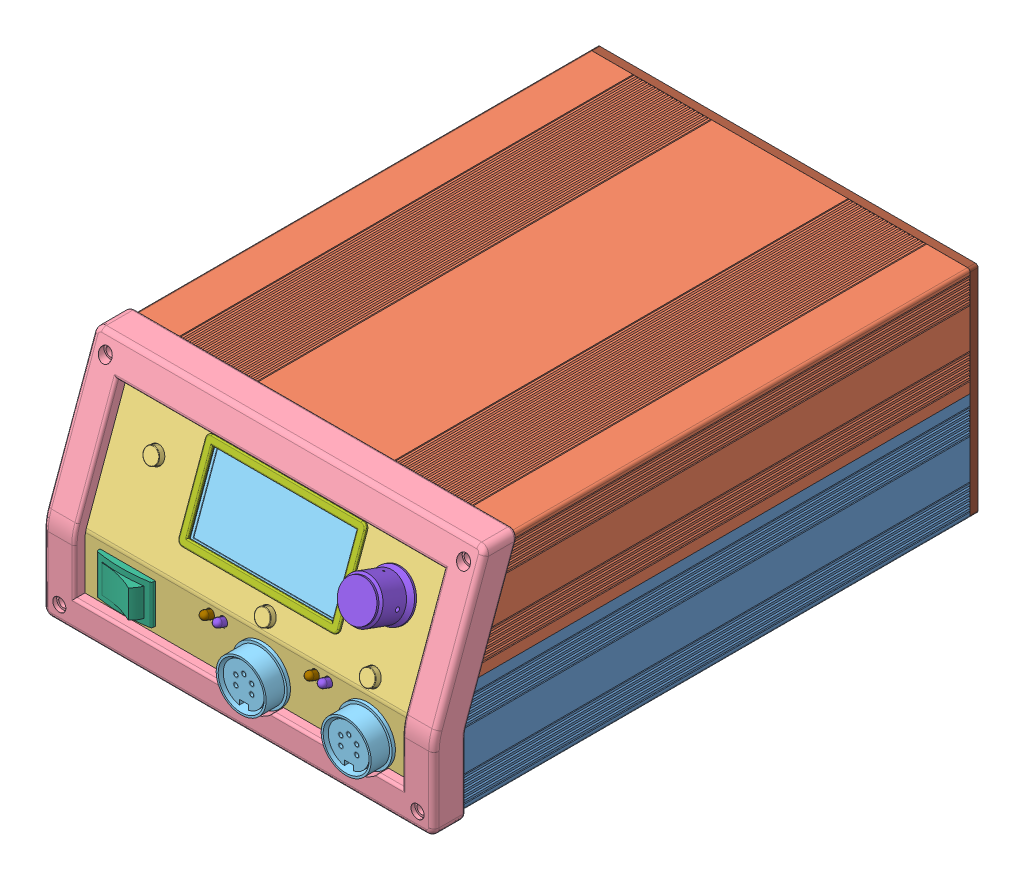
SolidWorks assembly Assembly, configuration Default. Lengths in mm. (continued)
Components (placement in the parent): (continued)
- SolderingStation-3: SolderingStation [Default] at (108 -45.1633 3.8854) x (-1 0 0) z (0 -0.34202 -0.939693) size (142.21 62 43.76) (continued)
  - SolderingStation.step-1: SolderingStation.step [Default] at origin size (142.21 62 43.76) (continued)
    - R10_ss.step-1: R10_ss.step [Default] at origin size (1.7 0.8 0.56)
      - User_Library-RES_1609-0603.step-1: User_Library-RES_1609-0603.step [Default] at (120.9541 53.774 0) x (1 0 0) z (0 -1 0) size (1.7 0.56 0.8)
    - R11_ss.step-1: R11_ss.step [Default] at origin size (0.8 1.7 0.56)
      - User_Library-RES_1609-0603.step-1: User_Library-RES_1609-0603.step [Default] at (79.298 51.2339 0) x (0 -1 0) z (-1 0 0) size (1.7 0.56 0.8)
    - R12_ss.step-1: R12_ss.step [Default] at origin size (0.8 1.7 0.56)
      - User_Library-RES_1609-0603.step-1: User_Library-RES_1609-0603.step [Default] at (118.7951 51.2339 0) x (0 -1 0) z (-1 0 0) size (1.7 0.56 0.8)
    - U3_ss.step-1: U3_ss.step [Default] at origin size (6.2 5 1.75)
      - User_Library-SOIC8_JEDEC_MS-012AA.step-1: User_Library-SOIC8_JEDEC_MS-012AA.step [Default] at (86.8348 63.0449 0) x (0 -1 0) z (-1 0 0) size (5 1.75 6.2)
    - C8_ss.step-1: C8_ss.step [Default] at origin size (1.6 0.8 0.3)
      - User_Library-0603_SMD_Capacitor.step-1: User_Library-0603_SMD_Capacitor.step [Default] at (89.7629 66.4487 0) x (1 0 0) z (0 -1 0) size (1.6 0.3 0.8)
    - C10_ss.step-1: C10_ss.step [Default] at origin size (1.6 0.8 0.3)
      - User_Library-0603_SMD_Capacitor.step-1: User_Library-0603_SMD_Capacitor.step [Default] at (85.2671 59.4891 0) x (1 0 0) z (0 -1 0) size (1.6 0.3 0.8)
    - D7_ss.step-1: D7_ss.step [Default] at origin size (2.5 3 1.1)
      - CircuitWorks-SOT-23.step-1: CircuitWorks-SOT-23.step [Default] at (79.4249 63.6799 0.5) x (0 -1 0) z (-1 0 0) size (3 1.1 2.5)
    - D3_ss.step-1: D3_ss.step [Default] at origin size (3 2.5 1.1)
      - CircuitWorks-SOT-23.step-1: CircuitWorks-SOT-23.step [Default] at (93.9031 63.8069 0.5) x (1 0 0) z (0 -1 0) size (3 1.1 2.5)
    - R13_ss.step-1: R13_ss.step [Default] at origin size (1.7 0.8 0.56)
      - User_Library-RES_1609-0603.step-1: User_Library-RES_1609-0603.step [Default] at (93.7759 66.474 0) x (-1 0 0) z (0 1 0) size (1.7 0.56 0.8)
    - R15_ss.step-1: R15_ss.step [Default] at origin size (0.8 1.7 0.56)
      - User_Library-RES_1609-0603.step-1: User_Library-RES_1609-0603.step [Default] at (96.57 65.7121 0) x (0 1 0) z (1 0 0) size (1.7 0.56 0.8)
    - R17_ss.step-1: R17_ss.step [Default] at origin size (0.8 1.7 0.56)
      - User_Library-RES_1609-0603.step-1: User_Library-RES_1609-0603.step [Default] at (96.57 62.7911 0) x (0 1 0) z (1 0 0) size (1.7 0.56 0.8)
    - R21_ss.step-1: R21_ss.step [Default] at origin size (0.8 1.7 0.56)
      - User_Library-RES_1609-0603.step-1: User_Library-RES_1609-0603.step [Default] at (91.1352 60.5051 0) x (0 1 0) z (1 0 0) size (1.7 0.56 0.8)
    - R22_ss.step-1: R22_ss.step [Default] at origin size (0.8 1.7 0.56)
      - User_Library-RES_1609-0603.step-1: User_Library-RES_1609-0603.step [Default] at (91.1352 63.0451 0) x (0 1 0) z (1 0 0) size (1.7 0.56 0.8)
    - R29_ss.step-1: R29_ss.step [Default] at origin size (1.7 0.8 0.56)
      - User_Library-RES_1609-0603.step-1: User_Library-RES_1609-0603.step [Default] at (79.8061 59.235 0) x (1 0 0) z (0 -1 0) size (1.7 0.56 0.8)
    - R31_ss.step-1: R31_ss.step [Default] at origin size (1.7 0.8 0.56)
      - User_Library-RES_1609-0603.step-1: User_Library-RES_1609-0603.step [Default] at (79.8061 60.632 0) x (1 0 0) z (0 -1 0) size (1.7 0.56 0.8)
    - R33_ss.step-1: R33_ss.step [Default] at origin size (0.8 1.7 0.56)
      - User_Library-RES_1609-0603.step-1: User_Library-RES_1609-0603.step [Default] at (82.0919 64.3151 0) x (0 1 0) z (1 0 0) size (1.7 0.56 0.8)
    - R35_ss.step-1: R35_ss.step [Default] at origin size (0.8 1.7 0.56)
      - User_Library-RES_1609-0603.step-1: User_Library-RES_1609-0603.step [Default] at (82.0919 61.7751 0) x (0 1 0) z (1 0 0) size (1.7 0.56 0.8)
    - R36_ss.step-1: R36_ss.step [Default] at origin size (0.8 1.7 0.56)
      - User_Library-RES_1609-0603.step-1: User_Library-RES_1609-0603.step [Default] at (121.97 61.7751 0) x (0 1 0) z (1 0 0) size (1.7 0.56 0.8)
    - R34_ss.step-1: R34_ss.step [Default] at origin size (0.8 1.7 0.56)
      - User_Library-RES_1609-0603.step-1: User_Library-RES_1609-0603.step [Default] at (121.97 64.3151 0) x (0 1 0) z (1 0 0) size (1.7 0.56 0.8)
    - R32_ss.step-1: R32_ss.step [Default] at origin size (1.7 0.8 0.56)
      - User_Library-RES_1609-0603.step-1: User_Library-RES_1609-0603.step [Default] at (119.8061 60.632 0) x (1 0 0) z (0 -1 0) size (1.7 0.56 0.8)
    - R30_ss.step-1: R30_ss.step [Default] at origin size (1.7 0.8 0.56)
      - User_Library-RES_1609-0603.step-1: User_Library-RES_1609-0603.step [Default] at (119.8061 59.235 0) x (1 0 0) z (0 -1 0) size (1.7 0.56 0.8)
    - R24_ss.step-1: R24_ss.step [Default] at origin size (0.8 1.7 0.56)
      - User_Library-RES_1609-0603.step-1: User_Library-RES_1609-0603.step [Default] at (131.0836 63.0451 0) x (0 1 0) z (1 0 0) size (1.7 0.56 0.8)
    - R23_ss.step-1: R23_ss.step [Default] at origin size (0.8 1.7 0.56)
      - User_Library-RES_1609-0603.step-1: User_Library-RES_1609-0603.step [Default] at (131.0885 60.5051 0) x (0 1 0) z (1 0 0) size (1.7 0.56 0.8)
    - R18_ss.step-1: R18_ss.step [Default] at origin size (0.8 1.7 0.56)
      - User_Library-RES_1609-0603.step-1: User_Library-RES_1609-0603.step [Default] at (136.5699 62.7911 0) x (0 1 0) z (1 0 0) size (1.7 0.56 0.8)
    - R16_ss.step-1: R16_ss.step [Default] at origin size (0.8 1.7 0.56)
      - User_Library-RES_1609-0603.step-1: User_Library-RES_1609-0603.step [Default] at (136.5699 65.7121 0) x (0 1 0) z (1 0 0) size (1.7 0.56 0.8)
    - R14_ss.step-1: R14_ss.step [Default] at origin size (1.7 0.8 0.56)
      - User_Library-RES_1609-0603.step-1: User_Library-RES_1609-0603.step [Default] at (133.7759 66.474 0) x (-1 0 0) z (0 1 0) size (1.7 0.56 0.8)
    - D4_ss.step-1: D4_ss.step [Default] at origin size (3 2.5 1.1)
      - CircuitWorks-SOT-23.step-1: CircuitWorks-SOT-23.step [Default] at (133.9031 63.8069 0.5) x (1 0 0) z (0 -1 0) size (3 1.1 2.5)
    - D8_ss.step-1: D8_ss.step [Default] at origin size (2.5 3 1.1)
      - CircuitWorks-SOT-23.step-1: CircuitWorks-SOT-23.step [Default] at (119.4299 63.6799 0.5) x (0 -1 0) z (-1 0 0) size (3 1.1 2.5)
    - C11_ss.step-1: C11_ss.step [Default] at origin size (1.6 0.8 0.3)
      - User_Library-0603_SMD_Capacitor.step-1: User_Library-0603_SMD_Capacitor.step [Default] at (125.2671 59.4891 0) x (1 0 0) z (0 -1 0) size (1.6 0.3 0.8)
    - C9_ss.step-1: C9_ss.step [Default] at origin size (1.6 0.8 0.3)
      - User_Library-0603_SMD_Capacitor.step-1: User_Library-0603_SMD_Capacitor.step [Default] at (129.6917 66.7027 0) x (1 0 0) z (0 -1 0) size (1.6 0.3 0.8)
    - U4_ss.step-1: U4_ss.step [Default] at origin size (6.2 5 1.75)
      - User_Library-SOIC8_JEDEC_MS-012AA.step-1: User_Library-SOIC8_JEDEC_MS-012AA.step [Default] at (126.8348 63.0449 0) x (0 -1 0) z (-1 0 0) size (5 1.75 6.2)
    - R44_ss.step-1: R44_ss.step [Default] at origin size (1.7 0.8 0.56)
      - User_Library-RES_1609-0603.step-1: User_Library-RES_1609-0603.step [Default] at (63.6769 67.1089 0) x (-1 0 0) z (0 1 0) size (1.7 0.56 0.8)
    - R46_ss.step-1: R46_ss.step [Default] at origin size (1.7 0.8 0.56)
      - User_Library-RES_1609-0603.step-1: User_Library-RES_1609-0603.step [Default] at (60.2481 67.109 0) x (1 0 0) z (0 -1 0) size (1.7 0.56 0.8)
    - FB1_ss.step-1: FB1_ss.step [Default] at origin size (1.25 2 0.85)
      - FB-0805.step-1: FB-0805.step [Default] at (55.5489 42.9791 0) x (0 1 0) z (0 0 1) size (2 1.25 0.85)
        - User_Library-FB_2012-1_Pad001.step-1: User_Library-FB_2012-1_Pad001.step [Default] at (0 0 0.03) size (1.94 1.19 0.79)
        - User_Library-FB_2012-1_Cut.step-1: User_Library-FB_2012-1_Cut.step [Default] at origin size (2 1.25 0.85)
    - FB2_ss.step-1: FB2_ss.step [Default] at origin size (1.25 2 0.85)
      - FB-0805.step-1: FB-0805.step [Default] at (95.6809 42.9791 0) x (0 1 0) z (0 0 1) size (2 1.25 0.85)
        - User_Library-FB_2012-1_Pad001.step-1: User_Library-FB_2012-1_Pad001.step [Default] at (0 0 0.03) size (1.94 1.19 0.79)
        - User_Library-FB_2012-1_Cut.step-1: User_Library-FB_2012-1_Cut.step [Default] at origin size (2 1.25 0.85)
    - Q3_ss.step-1: Q3_ss.step [Default] at origin size (2.5 3 1.1)
      - CircuitWorks-SOT-23.step-1: CircuitWorks-SOT-23.step [Default] at (84.7589 53.7739 0.5) x (0 -1 0) z (-1 0 0) size (3 1.1 2.5)
    - R54_ss.step-1: R54_ss.step [Default] at origin size (0.8 1.7 0.56)
      - User_Library-RES_1609-0603.step-1: User_Library-RES_1609-0603.step [Default] at (107.1649 60.9601 0) x (0 1 0) z (1 0 0) size (1.7 0.56 0.8)
    - R55_ss.step-1: R55_ss.step [Default] at origin size (0.8 1.7 0.56)
      - User_Library-RES_1609-0603.step-1: User_Library-RES_1609-0603.step [Default] at (113.007 60.9601 0) x (0 1 0) z (1 0 0) size (1.7 0.56 0.8)
    - U6_ss.step-1: U6_ss.step [Default] at origin size (2.4 2.2 1.1)
      - User_Library-SOT353-1.step-1: User_Library-SOT353-1.step [Default] at (104.879 60.9598 0) x (0 -1 0) z (0 0 1) size (2.2 2.4 1.1)
    - U7_ss.step-1: U7_ss.step [Default] at origin size (2.4 2.2 1.1)
      - User_Library-SOT353-1.step-1: User_Library-SOT353-1.step [Default] at (110.721 60.9598 0) x (0 -1 0) z (0 0 1) size (2.2 2.4 1.1)
    - D16_ss.step-1: D16_ss.step [Default] at origin size (3 2.5 1.1)
      - CircuitWorks-SOT-23.step-1: CircuitWorks-SOT-23.step [Default] at (112.3949 84.0741 0.5) x (-1 0 0) z (0 1 0) size (3 1.1 2.5)
    - R58_ss.step-1: R58_ss.step [Default] at origin size (1.7 0.8 0.56)
      - User_Library-RES_1609-0603.step-1: User_Library-RES_1609-0603.step [Default] at (105.3847 85.09 0) x (1 0 0) z (0 -1 0) size (1.7 0.56 0.8)
    - R59_ss.step-1: R59_ss.step [Default] at origin size (1.7 0.8 0.56)
      - User_Library-RES_1609-0603.step-1: User_Library-RES_1609-0603.step [Default] at (147.3701 81.1806 0) x (1 0 0) z (0 -1 0) size (1.7 0.56 0.8)
    - J1_ss.step-1: J1_ss.step [Default] at origin size (12.4 6.1 10.4)
      - User_Library-XH-A-4.step-1: User_Library-XH-A-4.step [Default] at (131.0403 87.3751 7) x (-1 0 0) z (0 0 1) size (12.4 6.1 10.4)
    - R60_ss.step-1: R60_ss.step [Default] at origin size (1.7 0.8 0.56)
      - User_Library-RES_1609-0603.step-1: User_Library-RES_1609-0603.step [Default] at (86.6639 66.474 0) x (-1 0 0) z (0 1 0) size (1.7 0.56 0.8)
    - R61_ss.step-1: R61_ss.step [Default] at origin size (1.7 0.8 0.56)
      - User_Library-RES_1609-0603.step-1: User_Library-RES_1609-0603.step [Default] at (126.5419 66.474 0) x (-1 0 0) z (0 1 0) size (1.7 0.56 0.8)
    - R62_ss.step-1: R62_ss.step [Default] at origin size (1.7 0.8 0.56)
      - User_Library-RES_1609-0603.step-1: User_Library-RES_1609-0603.step [Default] at (82.8539 66.474 0) x (-1 0 0) z (0 1 0) size (1.7 0.56 0.8)
    - R63_ss.step-1: R63_ss.step [Default] at origin size (1.7 0.8 0.56)
      - User_Library-RES_1609-0603.step-1: User_Library-RES_1609-0603.step [Default] at (122.7319 66.474 0) x (-1 0 0) z (0 1 0) size (1.7 0.56 0.8)
    - R65_ss.step-1: R65_ss.step [Default] at origin size (1.7 0.8 0.56)
      - User_Library-RES_1609-0603.step-1: User_Library-RES_1609-0603.step [Default] at (134.7193 83.3874 0) x (-1 0 0) z (0 1 0) size (1.7 0.56 0.8)
    - R66_ss.step-1: R66_ss.step [Default] at origin size (1.7 0.8 0.56)
      - User_Library-RES_1609-0603.step-1: User_Library-RES_1609-0603.step [Default] at (134.7193 82.1174 0) x (-1 0 0) z (0 1 0) size (1.7 0.56 0.8)
    - C19_ss.step-1: C19_ss.step [Default] at origin size (1.6 0.8 0.3)
      - User_Library-0603_SMD_Capacitor.step-1: User_Library-0603_SMD_Capacitor.step [Default] at (100.0761 56.8199 0) x (1 0 0) z (0 -1 0) size (1.6 0.3 0.8)
    - R67_ss.step-1: R67_ss.step [Default] at origin size (1.7 0.8 0.56)
      - User_Library-RES_1609-0603.step-1: User_Library-RES_1609-0603.step [Default] at (94.3609 56.769 0) x (-1 0 0) z (0 1 0) size (1.7 0.56 0.8)
    - R68_ss.step-1: R68_ss.step [Default] at origin size (0.8 1.7 0.56)
      - User_Library-RES_1609-0603.step-1: User_Library-RES_1609-0603.step [Default] at (103.4279 52.2501 0) x (0 1 0) z (1 0 0) size (1.7 0.56 0.8)
    - R69_ss.step-1: R69_ss.step [Default] at origin size (0.8 1.7 0.56)
      - User_Library-RES_1609-0603.step-1: User_Library-RES_1609-0603.step [Default] at (92.7861 51.7145 0) x (0 1 0) z (1 0 0) size (1.7 0.56 0.8)
    - R70_ss.step-1: R70_ss.step [Default] at origin size (0.8 1.7 0.56)
      - User_Library-RES_1609-0603.step-1: User_Library-RES_1609-0603.step [Default] at (102.158 52.2501 0) x (0 1 0) z (1 0 0) size (1.7 0.56 0.8)
    - U8_ss.step-1: U8_ss.step [Default] at origin size (6.2 5 1.75)
      - User_Library-SOIC8_JEDEC_MS-012AA.step-1: User_Library-SOIC8_JEDEC_MS-012AA.step [Default] at (97.6298 53.2659 0) x (0 -1 0) z (-1 0 0) size (5 1.75 6.2)
    - F1_ss.step-1: F1_ss.step [Default] at origin size (6.83 23.38 12.19)
      - User_Library-Clips_FC-201_with_fuse_5x20.step-1: User_Library-Clips_FC-201_with_fuse_5x20.step [Default] at (167.6415 46.9901 0.1) x (-1 0 0) z (0 0 1) size (6.83 23.38 12.19)
        - User_Library-Clips_FC-201_with_fuse_5x20_FC-201.step-1: User_Library-Clips_FC-201_with_fuse_5x20_FC-201.step [Default] at (0 -8.0775 0) size (6.83 7.22 12.19)
        - User_Library-Clips_FC-201_with_fuse_5x20_FC-201.step-2: User_Library-Clips_FC-201_with_fuse_5x20_FC-201.step [Default] at (0 8.0775 0) x (-1 0 0) z (0 0 1) size (6.83 7.22 12.19)
        - User_Library-Clips_FC-201_with_fuse_5x20_5x20.step-1: User_Library-Clips_FC-201_with_fuse_5x20_5x20.step [Default] at (0 0 5.715) x (-1 0 0) z (0 -1 0) size (5 5 20)
- Setback-3: Setback [Default] at (-32.5 21.11 -194.5) x (-1 0 0) z (0 0 -1) size (57 24 17.19)
  - Setback.step-1: Setback.step [Default] at origin size (57 24 17.19)
    - Board_sb.step-1: Board_sb.step [Default] at origin size (57 24 1.69)
      - Open CASCADE STEP translator 6.8 3.1.1.step-1: Open CASCADE STEP translator 6.8 3.1.1.step [Default] at (0 0 -1.6914) size (57 24 1.69)
    - F1_sb.step-1: F1_sb.step [Default] at origin size (1.46 2.1 0.71)
      - PTC_FUSE_0805.step-1: PTC_FUSE_0805.step [Default] at (-11.7 -5.3 -1.6914) x (0 -1 0) z (0 0 -1) size (2.1 1.45 0.71)
    - SP2_sb.step-1: SP2_sb.step [Default] at origin size (6 6 6)
      - 6mmSpacer.step-1: 6mmSpacer.step [Default] at (-24.9999 0.0001 0) x (1 0 0) z (0 -1 0) size (6 6 6)
    - SP1_sb.step-1: SP1_sb.step [Default] at origin size (6 6 6)
      - 6mmSpacer.step-1: 6mmSpacer.step [Default] at (25.0001 0.0001 0) x (1 0 0) z (0 -1 0) size (6 6 6)
    - J2_sb.step-1: J2_sb.step [Default] at origin size (16 16 10.5)
      - Mini-DIN-socket-3-pin.step-1: Mini-DIN-socket-3-pin.step [Default] at (9.9999 -0.0001 5) x (-1 0 0) z (0 1 0) size (16 10.5 16)
    - J1_sb.step-1: J1_sb.step [Default] at origin size (16 16 10.5)
      - Mini-DIN-socket-3-pin.step-1: Mini-DIN-socket-3-pin.step [Default] at (-10.0001 -0.0001 5) x (-1 0 0) z (0 1 0) size (16 10.5 16)
    - J3_sb.step-1: J3_sb.step [Default] at origin size (12.4 6.1 10.4)
      - User_Library-XH-A-4.step-1: User_Library-XH-A-4.step [Default] at (-6.2001 -8.6249 -8.6914) x (1 0 0) z (0 0 -1) size (12.4 6.1 10.4)
Mates (geometry in assembly coordinates):
- Coincident14: coincident aligned: line of CaseExtrusion-ModifiedBottom-4 through (1 -72.5 -39.1) axis (0 0 -1); line of Front Panel-1 through (-72.5 -12.3527 0) axis (0 -1 0)
- Coincident21: coincident anti-aligned: plane of Front Panel-1 through (-72.5 -12 2) normal (0 0 1); plane of AmphenolSocket-4 through (45 -25.1 2) normal (0 0 -1)
- Coincident22: coincident anti-aligned: plane of Front Panel-1 through (-72.5 -12 2) normal (0 0 1); plane of AmphenolSocket-3 through (5 -25.1 2) normal (0 0 -1)
- Concentric1: concentric aligned: circle of Front Panel-1; circle of AmphenolSocket-3
- Concentric2: concentric aligned: circle of Front Panel-1; circle of AmphenolSocket-4
- Coincident27: coincident anti-aligned: plane of CaseExtrusion-ModifiedBottom-4 through (69.25 -33.6 -200) normal (0 0 -1); plane of Rear Panel-1 through (71.5 -40.09 -200) normal (0 0 1)
- Coincident61: coincident anti-aligned: plane of CaseExtrusion-ModifiedBottom-4 through (-72.5 -41.1 -200) normal (-1 0 0); plane of Front Panel Bezel-1 through (-72.5 -10.7242 6) normal (1 0 0)
- Coincident62: coincident anti-aligned: plane of CaseExtrusion-ModifiedBottom-4 through (-72.5 -41.1 -160) normal (0 -1 0); plane of Front Panel Bezel-1 through (-164.7516 -41.1 2) normal (0 1 0)
- Coincident68: coincident anti-aligned: plane of Front Panel-1 through (-72.5 -12 2) normal (0 0 1); plane of RockerSwitch-1 through (-46.5075 -22.4992 2) normal (0 0 -1)
- Coincident77: coincident anti-aligned: plane of Front Panel-1 through (-72.5 -12 2) normal (0 0 1); plane of Front Panel Bezel-1 through (-164.7516 -41.1 2) normal (0 0 -1)
- Concentric7: concentric aligned: cylinder of Rear Panel-1 through (-62.5 -19.89 -203) axis (0 0 1) radius 1.525; circle of IEC_Connector_Fused_Flanges (Schurter 6200)-1
- Concentric8: concentric anti-aligned: cylinder of Rear Panel-1 through (-26.5 -19.89 -203) axis (0 0 1) radius 1.525; circle of IEC_Connector_Fused_Flanges (Schurter 6200)-1
- Coincident78: coincident: plane of Rear Panel-1 through (71.5 -40.09 -203) normal (0 0 -1); line of IEC_Connector_Fused_Flanges (Schurter 6200)-1 through (-32.511 -36.89 -203) axis (-1 0 0)
- Concentric12: concentric anti-aligned: circle of Triad Magnetics-VPT48-3300-1; circle of Transformer Mounting Plate-1
- Distance5: distance = 4 mm anti-aligned: plane of CaseExtrusion-ModifiedBottom-4 through (-4.3 -37.6 -200) normal (0 1 0); plane of Transformer Mounting Plate-1 through (0 -33.6 -100) normal (0 -1 0)
- Coincident80: coincident anti-aligned: plane of Triad Magnetics-VPT48-3300-1 through (31.8919 -31.6 -80.273) normal (0 -1 0); plane of Transformer Mounting Plate-1 through (0 -31.6 -100) normal (0 1 0)
- Concentric13: concentric aligned: circle of CaseExtrusion-ModifiedBottom-4; circle of Transformer Mounting Plate-1
- Concentric14: concentric aligned: circle of CaseExtrusion-ModifiedBottom-4; circle of Transformer Mounting Plate-1
- Coincident84: coincident anti-aligned: plane of Front Panel-1 through (-72.5 -16.2 2) normal (0 -1 0); plane of RockerSwitch-1 through (-46.5075 -16.2 -5.3533) normal (0 1 0)
- Coincident85: coincident anti-aligned: plane of Front Panel-1 through (-37.3 -12 2) normal (-1 0 0); plane of RockerSwitch-1 through (-37.3 -16.2 2) normal (1 0 0)
- Coincident86: coincident aligned: plane of CaseExtrusion-ModifiedBottom-4 through (69.25 -33.6 -200) normal (0 0 -1); plane of CaseExtrusion-ModifiedTop-7 through (-69.25 33.6 -200) normal (0 0 -1)
- Coincident87: coincident anti-aligned: plane of CaseExtrusion-ModifiedBottom-4 through (70 2 -200) normal (1 0 0); plane of CaseExtrusion-ModifiedTop-7 through (70 0 -200) normal (-1 0 0)
- Coincident88: coincident anti-aligned: plane of CaseExtrusion-ModifiedBottom-4 through (70 0 -200) normal (0 1 0); plane of CaseExtrusion-ModifiedTop-7 through (72.5 0 -200) normal (0 -1 0)
- Coincident89: coincident anti-aligned: plane of CaseExtrusion-ModifiedTop-7 through (-69.25 33.6 -200) normal (0 0 -1); plane of Rear Panel-1 through (71.5 -40.09 -200) normal (0 0 1)
- Coincident90: coincident aligned: circle of CaseExtrusion-ModifiedTop-7; cylinder of Rear Panel-1 through (-68.25 36.86 -203) axis (0 0 -1) radius 1.7
- Concentric19: concentric aligned: circle of CaseExtrusion-ModifiedTop-7; cylinder of Rear Panel-1 through (68.25 36.86 -203) axis (0 0 -1) radius 1.7
- Coincident95: coincident anti-aligned: plane of CaseExtrusion-ModifiedTop-7 through (0 -1.4037 -3.8567) normal (0 0.34202 0.939693); plane of Front Panel-1 through (-72.5 -12 0) normal (0 -0.34202 -0.939693)
- Parallel1: parallel anti-aligned: line of Front Panel Bezel-1 through (13.9198 -31.1 5) axis (1 0 0); line of AmphenolSocket-3 through (6.719 -30.8203 9.27) axis (-1 0 0)
- Parallel2: parallel anti-aligned: line of Front Panel Bezel-1 through (13.9198 -31.1 5) axis (1 0 0); line of AmphenolSocket-4 through (46.719 -30.8203 9.27) axis (-1 0 0)
- Distance7: distance = 2 mm aligned: plane of b32-2000-1 through (5 -4.5166 1.533) normal (0 0.34202 0.939693); plane of Front Panel-1 through (-72.5 -11.316 1.8794) normal (0 0.34202 0.939693)
- Distance8: distance = 2 mm aligned: plane of b32-2000-3 through (45 -4.5166 1.533) normal (0 0.34202 0.939693); plane of Front Panel-1 through (-72.5 -11.316 1.8794) normal (0 0.34202 0.939693)
- Concentric24: concentric aligned: circle of Front Panel-1; circle of b32-2000-3
- Concentric25: concentric aligned: circle of Front Panel-1; circle of b32-2000-1
- Distance10: distance = 2 mm aligned: plane of b32-2000-4 through (-35.0175 18.0147 -6.6678) normal (0 0.34202 0.939693); plane of Front Panel-1 through (-72.5 -11.316 1.8794) normal (0 0.34202 0.939693)
- Coincident96: coincident anti-aligned: plane of Rear Panel-1 through (71.5 -40.09 -200) normal (0 0 1); plane of User Library-3.5MM Panel Mount Audio Jack - 3 Connector-1/User Library-3.5MM Panel Mount Audio Jack - 3 Connector_3.5MM Panel Mount Audio Jack - 4 Connector - korpus-1 through (-30.85 21.11 -200) normal (0 0 -1)
- Concentric29: concentric anti-aligned: circle of Rear Panel-1; circle of User Library-3.5MM Panel Mount Audio Jack - 3 Connector-1/User Library-3.5MM Panel Mount Audio Jack - 3 Connector_3.5MM Panel Mount Audio Jack - 4 Connector - korpus-1
- Concentric30: concentric aligned: circle of Front Panel-1; circle of Knob-1
- Distance12: distance = 2 mm anti-aligned: plane of Knob-1 through (54.7313 17.0964 -6.3335) normal (0 -0.34202 -0.939693); plane of Front Panel-1 through (-72.5 -11.316 1.8794) normal (0 0.34202 0.939693)
- Concentric33: concentric aligned: cylinder of Front Panel-1 through (68.25 -36.85 0) axis (0 0 1) radius 1.25; cylinder of Front Panel Bezel #2-2 through (68.25 -36.85 -25.8297) axis (0 0 1) radius 1.75
- Concentric34: concentric aligned: cylinder of Front Panel-1 through (-68.25 -36.85 0) axis (0 0 1) radius 1.25; cylinder of Front Panel Bezel #2-2 through (-68.25 -36.85 -25.8297) axis (0 0 1) radius 1.75
- Coincident102: coincident anti-aligned: plane of Front Panel-1 through (-72.5 -11.316 1.8794) normal (0 0.34202 0.939693); plane of Front Panel Bezel #2-2 through (162.2446 -12.5 2.3103) normal (0 -0.34202 -0.939693)
- Coincident106: coincident anti-aligned: plane of Front Panel-1 through (-29.55 18.4227 -40.9913) normal (1 0 0); plane of OledBezel-3 through (-29.55 -1.5526 -3.8025) normal (-1 0 0)
- Coincident107: coincident anti-aligned: plane of Front Panel-1 through (-29.55 -11.1682 -30.2211) normal (0 0.939693 -0.34202); plane of OledBezel-3 through (29.55 -1.5526 -3.8025) normal (0 -0.939693 0.34202)
- Concentric36: concentric anti-aligned: cylinder of Rear Panel-1 through (-50.85 21.11 -203) axis (0 0 1) radius 7.5; circle of SolderingStationSetback-1/SolderingStationSetback.step-1/J1.step-1/Jack_3.5mm.step-1
- Coincident109: coincident anti-aligned: plane of Rear Panel-1 through (71.5 -40.09 -200) normal (0 0 1); plane of SolderingStationSetback-1/SolderingStationSetback.step-1/J1.step-1/Jack_3.5mm.step-1 through (-52.697 24.3139 -200) normal (0 0 -1)
- Concentric37: concentric aligned: cylinder of Front Panel-1 through (-50 37.0856 -15.7373) axis (0 0.34202 0.939693) radius 1.2; cylinder of SolderingStation-1 through (-50 34.3494 -23.2549) axis (0 0.34202 0.939693) radius 1.025
- Concentric38: concentric aligned: cylinder of Front Panel-1 through (50 37.0856 -15.7373) axis (0 0.34202 0.939693) radius 1.2; cylinder of SolderingStation-1 through (50 34.3494 -23.2549) axis (0 0.34202 0.939693) radius 1.025
- Distance13: distance = 6 mm anti-aligned: plane of Front Panel-1 through (-72.5 -12 0) normal (0 -0.34202 -0.939693); plane of SolderingStation-1 through (62 -13.5749 -5.8118) normal (0 0.34202 0.939693)
- Concentric43: concentric aligned: cylinder of Front Panel-1 through (50 37.0856 -15.7373) axis (0 0.34202 0.939693) radius 1.2; cylinder of SolderingStation-3/SolderingStation.step-1/Board_ss.step-1/Open CASCADE STEP translator 6.8 4.1.1.step-1 through (50 34.3494 -23.2549) axis (0 0.34202 0.939693) radius 1.025
- Concentric44: concentric aligned: cylinder of Front Panel-1 through (-50 37.0856 -15.7373) axis (0 0.34202 0.939693) radius 1.2; cylinder of SolderingStation-3/SolderingStation.step-1/Board_ss.step-1/Open CASCADE STEP translator 6.8 4.1.1.step-1 through (-50 34.3494 -23.2549) axis (0 0.34202 0.939693) radius 1.025
- Distance16: distance = 6 mm anti-aligned: plane of SolderingStation-3/SolderingStation.step-1/Board_ss.step-1/Open CASCADE STEP translator 6.8 4.1.1.step-1 through (62 -13.5749 -5.8118) normal (0 0.34202 0.939693); plane of Front Panel-1 through (-72.5 -12 0) normal (0 -0.34202 -0.939693)
- Concentric45: concentric aligned: cylinder of Rear Panel-1 through (-57.5 21.11 -203) axis (0 0 1) radius 1.5; cylinder of Setback-3/Setback.step-1/Board_sb.step-1/Open CASCADE STEP translator 6.8 3.1.1.step-1 through (-57.5 21.11 -192.8086) axis (0 0 1) radius 1.025
- Concentric46: concentric aligned: cylinder of Rear Panel-1 through (-7.5 21.11 -203) axis (0 0 1) radius 1.5; cylinder of Setback-3/Setback.step-1/Board_sb.step-1/Open CASCADE STEP translator 6.8 3.1.1.step-1 through (-7.5 21.11 -192.8086) axis (0 0 1) radius 1.025
- Distance17: distance = 5.5 mm anti-aligned: plane of Setback-3/Setback.step-1/Board_sb.step-1/Open CASCADE STEP translator 6.8 3.1.1.step-1 through (-4 6.11 -194.5) normal (0 0 -1); plane of Rear Panel-1 through (71.5 -40.09 -200) normal (0 0 1)
